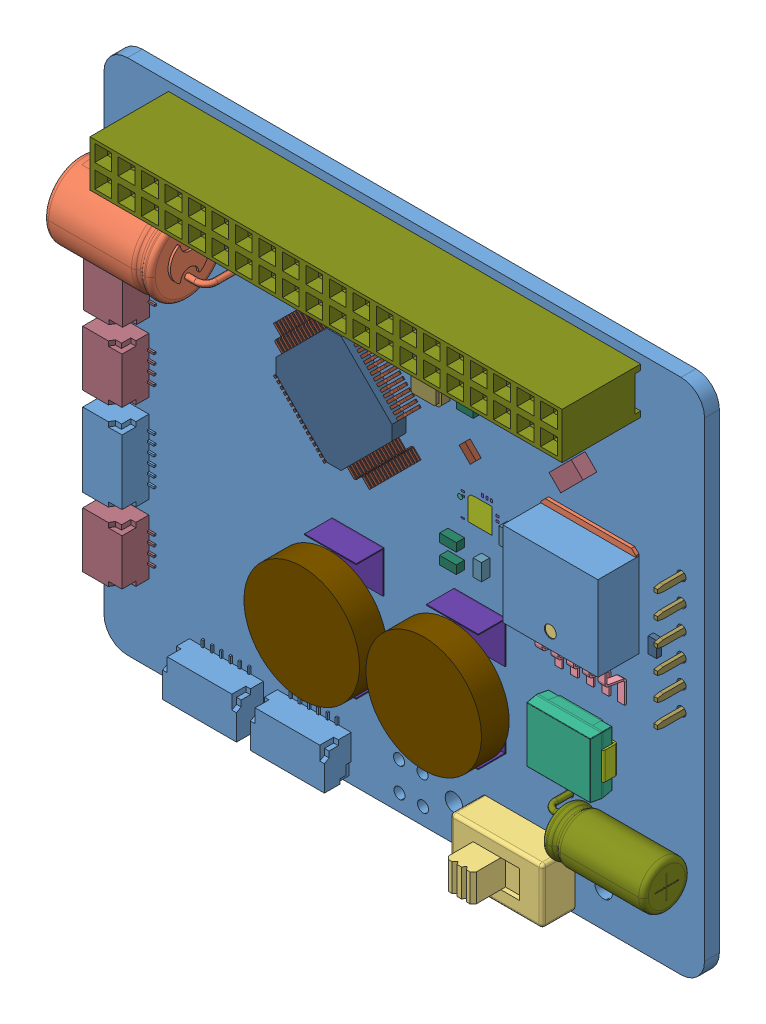
SolidWorks assembly FC_PiHat_REV1, configuration Default. Lengths in mm.
Overall size (65 56 12.01).
297 component instances, 38 part files, 0 mates.
Components (placement in the parent):
- FC_PiHat_REV1.step-1: FC_PiHat_REV1.step [Default] at origin size (65 56 12.01)
  - J7FC_PiHat_REV1.step-1: J7FC_PiHat_REV1.step [Default] at origin size (8 4.95 2.96)
    - SM06B-SRSS-TB.step-1: SM06B-SRSS-TB.step [Default] at (13.3 4.6 -0.3) x (1 0 0) z (0 -1 0) size (8 2.96 4.95)
  - C10FC_PiHat_REV1.step-1: C10FC_PiHat_REV1.step [Default] at origin size (13.96 8.06 10.04)
    - User_Library-Cap_electro_8x11_5x3_5mm_RA.step-1: User_Library-Cap_electro_8x11_5x3_5mm_RA.step [Default] at (13.5254 44.5 4) x (0 1 0) z (0 0 1) size (8.06 13.96 10.04)
  - J11FC_PiHat_REV1.step-1: J11FC_PiHat_REV1.step [Default] at origin size (10 6 9.8)
    - User_Library-EG1940-ND.step-1: User_Library-EG1940-ND.step [Default] at (40.9499 0.2249 0) x (1 0 0) z (0 0 1) size (10 6 9.8)
  - D4FC_PiHat_REV1.step-1: D4FC_PiHat_REV1.step [Default] at origin size (3.4 2.8 1.85)
    - User_Library-RGB_LED_Zwart_ASMT-YTC2-0AA02.step-1: User_Library-RGB_LED_Zwart_ASMT-YTC2-0AA02.step [Default] at (2.2908 8.9737 -1.6023) x (-1 0 0) z (0 -1 0) size (3.4 1.85 2.8)
      - Pootje_RGB_LED.step-1: Pootje_RGB_LED.step [Default] at (-0.3594 -0.1975 0.3238) size (0.9 1.1 0.5)
      - ASMT-YTC2-0AA02.step-1: ASMT-YTC2-0AA02.step [Default] at (-2.6594 -0.3475 0.5738) size (3 1.8 2.8)
      - Pootje_RGB_LED.step-2: Pootje_RGB_LED.step [Default] at (-0.3594 -0.1975 -0.5762) size (0.9 1.1 0.5)
      - Pootje_RGB_LED.step-3: Pootje_RGB_LED.step [Default] at (-0.3594 -0.1975 -1.4762) size (0.9 1.1 0.5)
      - Pootje_RGB_LED.step-4: Pootje_RGB_LED.step [Default] at (-1.9594 -0.1975 -1.9762) x (-1 0 0) z (0 0 -1) size (0.9 1.1 0.5)
      - Pootje_RGB_LED.step-5: Pootje_RGB_LED.step [Default] at (-1.9594 -0.1975 -1.0762) x (-1 0 0) z (0 0 -1) size (0.9 1.1 0.5)
      - Pootje_RGB_LED.step-6: Pootje_RGB_LED.step [Default] at (-1.9594 -0.1975 -0.1762) x (-1 0 0) z (0 0 -1) size (0.9 1.1 0.5)
  - D3FC_PiHat_REV1.step-1: D3FC_PiHat_REV1.step [Default] at origin size (3.4 2.8 1.85)
    - User_Library-RGB_LED_Zwart_ASMT-YTC2-0AA02.step-1: User_Library-RGB_LED_Zwart_ASMT-YTC2-0AA02.step [Default] at (2.3908 45.4737 -1.6023) x (-1 0 0) z (0 -1 0) size (3.4 1.85 2.8)
      - Pootje_RGB_LED.step-1: Pootje_RGB_LED.step [Default] at (-0.3594 -0.1975 0.3238) size (0.9 1.1 0.5)
      - ASMT-YTC2-0AA02.step-1: ASMT-YTC2-0AA02.step [Default] at (-2.6594 -0.3475 0.5738) size (3 1.8 2.8)
      - Pootje_RGB_LED.step-2: Pootje_RGB_LED.step [Default] at (-0.3594 -0.1975 -0.5762) size (0.9 1.1 0.5)
      - Pootje_RGB_LED.step-3: Pootje_RGB_LED.step [Default] at (-0.3594 -0.1975 -1.4762) size (0.9 1.1 0.5)
      - Pootje_RGB_LED.step-4: Pootje_RGB_LED.step [Default] at (-1.9594 -0.1975 -1.9762) x (-1 0 0) z (0 0 -1) size (0.9 1.1 0.5)
      - Pootje_RGB_LED.step-5: Pootje_RGB_LED.step [Default] at (-1.9594 -0.1975 -1.0762) x (-1 0 0) z (0 0 -1) size (0.9 1.1 0.5)
      - Pootje_RGB_LED.step-6: Pootje_RGB_LED.step [Default] at (-1.9594 -0.1975 -0.1762) x (-1 0 0) z (0 0 -1) size (0.9 1.1 0.5)
  - D2FC_PiHat_REV1.step-1: D2FC_PiHat_REV1.step [Default] at origin size (3.4 2.8 1.85)
    - User_Library-RGB_LED_Zwart_ASMT-YTC2-0AA02.step-1: User_Library-RGB_LED_Zwart_ASMT-YTC2-0AA02.step [Default] at (62.5092 10.7763 -1.6023) x (1 0 0) z (0 1 0) size (3.4 1.85 2.8)
      - Pootje_RGB_LED.step-1: Pootje_RGB_LED.step [Default] at (-0.3594 -0.1975 0.3238) size (0.9 1.1 0.5)
      - ASMT-YTC2-0AA02.step-1: ASMT-YTC2-0AA02.step [Default] at (-2.6594 -0.3475 0.5738) size (3 1.8 2.8)
      - Pootje_RGB_LED.step-2: Pootje_RGB_LED.step [Default] at (-0.3594 -0.1975 -0.5762) size (0.9 1.1 0.5)
      - Pootje_RGB_LED.step-3: Pootje_RGB_LED.step [Default] at (-0.3594 -0.1975 -1.4762) size (0.9 1.1 0.5)
      - Pootje_RGB_LED.step-4: Pootje_RGB_LED.step [Default] at (-1.9594 -0.1975 -1.9762) x (-1 0 0) z (0 0 -1) size (0.9 1.1 0.5)
      - Pootje_RGB_LED.step-5: Pootje_RGB_LED.step [Default] at (-1.9594 -0.1975 -1.0762) x (-1 0 0) z (0 0 -1) size (0.9 1.1 0.5)
      - Pootje_RGB_LED.step-6: Pootje_RGB_LED.step [Default] at (-1.9594 -0.1975 -0.1762) x (-1 0 0) z (0 0 -1) size (0.9 1.1 0.5)
  - D1FC_PiHat_REV1.step-1: D1FC_PiHat_REV1.step [Default] at origin size (3.4 2.8 1.85)
    - User_Library-RGB_LED_Zwart_ASMT-YTC2-0AA02.step-1: User_Library-RGB_LED_Zwart_ASMT-YTC2-0AA02.step [Default] at (62.7592 46.4263 -1.6023) x (1 0 0) z (0 1 0) size (3.4 1.85 2.8)
      - Pootje_RGB_LED.step-1: Pootje_RGB_LED.step [Default] at (-0.3594 -0.1975 0.3238) size (0.9 1.1 0.5)
      - ASMT-YTC2-0AA02.step-1: ASMT-YTC2-0AA02.step [Default] at (-2.6594 -0.3475 0.5738) size (3 1.8 2.8)
      - Pootje_RGB_LED.step-2: Pootje_RGB_LED.step [Default] at (-0.3594 -0.1975 -0.5762) size (0.9 1.1 0.5)
      - Pootje_RGB_LED.step-3: Pootje_RGB_LED.step [Default] at (-0.3594 -0.1975 -1.4762) size (0.9 1.1 0.5)
      - Pootje_RGB_LED.step-4: Pootje_RGB_LED.step [Default] at (-1.9594 -0.1975 -1.9762) x (-1 0 0) z (0 0 -1) size (0.9 1.1 0.5)
      - Pootje_RGB_LED.step-5: Pootje_RGB_LED.step [Default] at (-1.9594 -0.1975 -1.0762) x (-1 0 0) z (0 0 -1) size (0.9 1.1 0.5)
      - Pootje_RGB_LED.step-6: Pootje_RGB_LED.step [Default] at (-1.9594 -0.1975 -0.1762) x (-1 0 0) z (0 0 -1) size (0.9 1.1 0.5)
  - S1FC_PiHat_REV1.step-1: S1FC_PiHat_REV1.step [Default] at origin size (4.1 4.1 0.81)
    - 5843174976.step-1: 5843174976.step [Default] at (40.7 32.3 0) size (4.1 4.1 0.81)
      - Body.step-1: Body.step [Default] at (-2.05 -2.05 0)
        - Open_CASCADE_STEP_translator_6.8_14.2.1.x_t-1: Open_CASCADE_STEP_translator_6.8_14.2.1.x_t [Default] at origin
      - Open_CASCADE_STEP_translator_6.8_14.1.step-1: Open_CASCADE_STEP_translator_6.8_14.1.step [Default] at (-2.05 -2.05 0) size (0.52 0.52 0.01)
      - Thermal_Shape.step-1: Thermal_Shape.step [Default] at (-1.3 -1.35 -0.001) size (2.6 2.7 0)
      - Pin_Shape.step-1: Pin_Shape.step [Default] at (-2.05 -1.37 0) size (0.35 0.24 0)
      - Pin_Shape.step-2: Pin_Shape.step [Default] at (2.05 1.37 0) x (-1 0 0) z (0 0 1) size (0.35 0.24 0)
      - Pin_Shape.step-3: Pin_Shape.step [Default] at (-2.05 -0.87 0) size (0.35 0.24 0)
      - Pin_Shape.step-4: Pin_Shape.step [Default] at (2.05 0.87 0) x (-1 0 0) z (0 0 1) size (0.35 0.24 0)
      - Pin_Shape.step-5: Pin_Shape.step [Default] at (-2.05 -0.37 0) size (0.35 0.24 0)
      - Pin_Shape.step-6: Pin_Shape.step [Default] at (2.05 0.37 0) x (-1 0 0) z (0 0 1) size (0.35 0.24 0)
      - Pin_Shape.step-7: Pin_Shape.step [Default] at (-2.05 0.13 0) size (0.35 0.24 0)
      - Pin_Shape.step-8: Pin_Shape.step [Default] at (2.05 -0.13 0) x (-1 0 0) z (0 0 1) size (0.35 0.24 0)
      - Pin_Shape.step-9: Pin_Shape.step [Default] at (-2.05 0.63 0) size (0.35 0.24 0)
      - Pin_Shape.step-10: Pin_Shape.step [Default] at (2.05 -0.63 0) x (-1 0 0) z (0 0 1) size (0.35 0.24 0)
      - Pin_Shape.step-11: Pin_Shape.step [Default] at (-2.05 1.13 0) size (0.35 0.24 0)
      - Pin_Shape.step-12: Pin_Shape.step [Default] at (2.05 -1.13 0) x (-1 0 0) z (0 0 1) size (0.35 0.24 0)
      - Pin_Shape.step-13: Pin_Shape.step [Default] at (-1.13 -2.05 0) x (0 1 0) z (0 0 1) size (0.35 0.24 0)
      - Pin_Shape.step-14: Pin_Shape.step [Default] at (1.13 2.05 0) x (0 -1 0) z (0 0 1) size (0.35 0.24 0)
      - Pin_Shape.step-15: Pin_Shape.step [Default] at (-0.63 -2.05 0) x (0 1 0) z (0 0 1) size (0.35 0.24 0)
      - Pin_Shape.step-16: Pin_Shape.step [Default] at (0.63 2.05 0) x (0 -1 0) z (0 0 1) size (0.35 0.24 0)
      - Pin_Shape.step-17: Pin_Shape.step [Default] at (-0.13 -2.05 0) x (0 1 0) z (0 0 1) size (0.35 0.24 0)
      - Pin_Shape.step-18: Pin_Shape.step [Default] at (0.13 2.05 0) x (0 -1 0) z (0 0 1) size (0.35 0.24 0)
      - Pin_Shape.step-19: Pin_Shape.step [Default] at (0.37 -2.05 0) x (0 1 0) z (0 0 1) size (0.35 0.24 0)
      - Pin_Shape.step-20: Pin_Shape.step [Default] at (-0.37 2.05 0) x (0 -1 0) z (0 0 1) size (0.35 0.24 0)
      - Pin_Shape.step-21: Pin_Shape.step [Default] at (0.87 -2.05 0) x (0 1 0) z (0 0 1) size (0.35 0.24 0)
      - Pin_Shape.step-22: Pin_Shape.step [Default] at (-0.87 2.05 0) x (0 -1 0) z (0 0 1) size (0.35 0.24 0)
      - Pin_Shape.step-23: Pin_Shape.step [Default] at (1.37 -2.05 0) x (0 1 0) z (0 0 1) size (0.35 0.24 0)
      - Pin_Shape.step-24: Pin_Shape.step [Default] at (-1.37 2.05 0) x (0 -1 0) z (0 0 1) size (0.35 0.24 0)
  - R14FC_PiHat_REV1.step-1: R14FC_PiHat_REV1.step [Default] at origin size (1.7 0.9 0.55)
    - 6063442624.step-1: 6063442624.step [Default] at (8.7742 7.9 -2.1523) size (1.7 0.9 0.55)
      - Extruded.step-1: Extruded.step [Default] at origin size (1.7 0.9 0.55)
  - R13FC_PiHat_REV1.step-1: R13FC_PiHat_REV1.step [Default] at origin size (1.7 0.9 0.55)
    - 6063442624.step-1: 6063442624.step [Default] at (8.7742 9.8048 -2.1523) size (1.7 0.9 0.55)
      - Extruded.step-1: Extruded.step [Default] at origin size (1.7 0.9 0.55)
  - R12FC_PiHat_REV1.step-1: R12FC_PiHat_REV1.step [Default] at origin size (1.7 0.9 0.55)
    - 6063442624.step-1: 6063442624.step [Default] at (8.7742 11.7 -2.1523) size (1.7 0.9 0.55)
      - Extruded.step-1: Extruded.step [Default] at origin size (1.7 0.9 0.55)
  - R11FC_PiHat_REV1.step-1: R11FC_PiHat_REV1.step [Default] at origin size (1.7 0.9 0.55)
    - 6063442624.step-1: 6063442624.step [Default] at (9.05 44.4 -2.1523) size (1.7 0.9 0.55)
      - Extruded.step-1: Extruded.step [Default] at origin size (1.7 0.9 0.55)
  - R10FC_PiHat_REV1.step-1: R10FC_PiHat_REV1.step [Default] at origin size (1.7 0.9 0.55)
    - 6063442624.step-1: 6063442624.step [Default] at (9.05 46.3 -2.1523) size (1.7 0.9 0.55)
      - Extruded.step-1: Extruded.step [Default] at origin size (1.7 0.9 0.55)
  - R9FC_PiHat_REV1.step-1: R9FC_PiHat_REV1.step [Default] at origin size (0.9 1.7 0.55)
    - 6063442432.step-1: 6063442432.step [Default] at (59.9 29.7 0) size (0.9 1.7 0.55)
      - Extruded-0.step-1: Extruded-0.step [Default] at origin size (0.9 1.7 0.55)
  - R8FC_PiHat_REV1.step-1: R8FC_PiHat_REV1.step [Default] at origin size (1.7 0.9 0.55)
    - 6063442624.step-1: 6063442624.step [Default] at (9.05 48.2 -2.1523) size (1.7 0.9 0.55)
      - Extruded.step-1: Extruded.step [Default] at origin size (1.7 0.9 0.55)
  - R7FC_PiHat_REV1.step-1: R7FC_PiHat_REV1.step [Default] at origin size (1.84 1.84 0.55)
    - 6063441088.step-1: 6063441088.step [Default] at (39.9 37.9 0) size (1.84 1.84 0.55)
      - Extruded-1.step-1: Extruded-1.step [Default] at origin size (1.84 1.84 0.55)
  - R6FC_PiHat_REV1.step-1: R6FC_PiHat_REV1.step [Default] at origin size (1.7 0.9 0.55)
    - 6063442624.step-1: 6063442624.step [Default] at (56.2 11.8 -2.1523) size (1.7 0.9 0.55)
      - Extruded.step-1: Extruded.step [Default] at origin size (1.7 0.9 0.55)
  - R5FC_PiHat_REV1.step-1: R5FC_PiHat_REV1.step [Default] at origin size (1.7 0.9 0.55)
    - 6063442624.step-1: 6063442624.step [Default] at (56.2 10 -2.1523) size (1.7 0.9 0.55)
      - Extruded.step-1: Extruded.step [Default] at origin size (1.7 0.9 0.55)
  - R4FC_PiHat_REV1.step-1: R4FC_PiHat_REV1.step [Default] at origin size (1.7 0.9 0.55)
    - 6063442624.step-1: 6063442624.step [Default] at (56.2 8.2 -2.1523) size (1.7 0.9 0.55)
      - Extruded.step-1: Extruded.step [Default] at origin size (1.7 0.9 0.55)
  - R3FC_PiHat_REV1.step-1: R3FC_PiHat_REV1.step [Default] at origin size (1.7 0.9 0.55)
    - 6063442624.step-1: 6063442624.step [Default] at (56.8 47.4 -2.1523) size (1.7 0.9 0.55)
      - Extruded.step-1: Extruded.step [Default] at origin size (1.7 0.9 0.55)
  - R2FC_PiHat_REV1.step-1: R2FC_PiHat_REV1.step [Default] at origin size (1.7 0.9 0.55)
    - 6063442624.step-1: 6063442624.step [Default] at (56.8 45.6 -2.1523) size (1.7 0.9 0.55)
      - Extruded.step-1: Extruded.step [Default] at origin size (1.7 0.9 0.55)
  - R1FC_PiHat_REV1.step-1: R1FC_PiHat_REV1.step [Default] at origin size (1.7 0.9 0.55)
    - 6063442624.step-1: 6063442624.step [Default] at (56.8 43.8 -2.1523) size (1.7 0.9 0.55)
      - Extruded.step-1: Extruded.step [Default] at origin size (1.7 0.9 0.55)
  - J8FC_PiHat_REV1.step-1: J8FC_PiHat_REV1.step [Default] at origin size (4.95 8 2.96)
    - SM06B-SRSS-TB.step-1: SM06B-SRSS-TB.step [Default] at (4.55 19.8 -0.3) x (0 -1 0) z (-1 0 0) size (8 2.96 4.95)
  - J6FC_PiHat_REV1.step-1: J6FC_PiHat_REV1.step [Default] at origin size (10.06 15.53 5.7)
    - female_header_a-bl254-ea-g02d.step-1: female_header_a-bl254-ea-g02d.step [Default] at (61.2001 31.0851 -1.6023) x (0 -1 0) z (0 0 -1) size (5.33 10.06 5.7)
    - female_header_a-bl254-ea-g02d.step-2: female_header_a-bl254-ea-g02d.step [Default] at (61.2001 26.0099 -1.6023) x (0 -1 0) z (0 0 -1) size (5.33 10.06 5.7)
    - female_header_a-bl254-ea-g02d.step-3: female_header_a-bl254-ea-g02d.step [Default] at (61.2001 36.2099 -1.6023) x (0 -1 0) z (0 0 -1) size (5.33 10.06 5.7)
  - J4FC_PiHat_REV1.step-1: J4FC_PiHat_REV1.step [Default] at origin size (4.95 6 2.96)
    - SM04B-SRSS-TB.step-1: SM04B-SRSS-TB.step [Default] at (4.55 28.375 -0.3) x (0 -1 0) z (-1 0 0) size (6 2.96 4.95)
  - J3FC_PiHat_REV1.step-1: J3FC_PiHat_REV1.step [Default] at origin size (4.95 6 2.96)
    - SM04B-SRSS-TB.step-1: SM04B-SRSS-TB.step [Default] at (4.55 11.35 -0.3) x (0 -1 0) z (-1 0 0) size (6 2.96 4.95)
  - J2FC_PiHat_REV1.step-1: J2FC_PiHat_REV1.step [Default] at origin size (8 4.95 2.96)
    - SM06B-SRSS-TB.step-1: SM06B-SRSS-TB.step [Default] at (22.8093 4.575 -0.3) x (1 0 0) z (0 -1 0) size (8 2.96 4.95)
  - J1FC_PiHat_REV1.step-1: J1FC_PiHat_REV1.step [Default] at origin size (4.95 6 2.96)
    - SM04B-SRSS-TB.step-1: SM04B-SRSS-TB.step [Default] at (4.625 35.925 -0.3) x (0 -1 0) z (-1 0 0) size (6 2.96 4.95)
  - C4FC_PiHat_REV1.step-1: C4FC_PiHat_REV1.step [Default] at origin size (0.9 1.8 0.9)
    - 6063440896.step-1: 6063440896.step [Default] at (41.3 27.825 0) size (0.9 1.8 0.9)
      - Extruded-2.step-1: Extruded-2.step [Default] at origin size (0.9 1.8 0.9)
  - C3FC_PiHat_REV1.step-1: C3FC_PiHat_REV1.step [Default] at origin size (0.9 1.8 0.9)
    - 6063440896.step-1: 6063440896.step [Default] at (44.1 32.225 0) size (0.9 1.8 0.9)
      - Extruded-2.step-1: Extruded-2.step [Default] at origin size (0.9 1.8 0.9)
  - C2FC_PiHat_REV1.step-1: C2FC_PiHat_REV1.step [Default] at origin size (1.8 0.9 0.9)
    - 6063441280.step-1: 6063441280.step [Default] at (38.125 28.8 0) size (1.8 0.9 0.9)
      - Extruded-3.step-1: Extruded-3.step [Default] at origin size (1.8 0.9 0.9)
  - C1FC_PiHat_REV1.step-1: C1FC_PiHat_REV1.step [Default] at origin size (1.8 0.9 0.9)
    - 6063441280.step-1: 6063441280.step [Default] at (38.125 26.7 0) size (1.8 0.9 0.9)
      - Extruded-3.step-1: Extruded-3.step [Default] at origin size (1.8 0.9 0.9)
  - J5FC_PiHat_REV1.step-1: J5FC_PiHat_REV1.step [Default] at origin size (51.1 5 11.1)
    - User_Library-Header_2x20_2_54mm.step-1: User_Library-Header_2x20_2_54mm.step [Default] at (56.6601 52.5601 0) x (1 0 0) z (0 -1 0) size (51.1 11.1 5)
  - L2FC_PiHat_REV1.step-1: L2FC_PiHat_REV1.step [Default] at origin size (12.5 12.7 6.1)
    - 5843174592.step-1: 5843174592.step [Default] at (40.7 17.6 0) x (0 1 0) z (0 0 1) size (12.7 12.5 6.1)
      - pin.step-1: pin.step [Default] at (6.35 2.8 0) x (-1 0 0) z (0 0 1) size (4.5 5.6 3)
        - Open_CASCADE_STEP_translator_6.8_3.3.1.step-1: Open_CASCADE_STEP_translator_6.8_3.3.1.step [Default] at origin size (4.5 5.6 3)
      - pin.step-2: pin.step [Default] at (-6.35 -2.8 0) size (4.5 5.6 3)
        - Open_CASCADE_STEP_translator_6.8_3.3.1.step-1: Open_CASCADE_STEP_translator_6.8_3.3.1.step [Default] at origin size (4.5 5.6 3)
      - Body.step-1: Body.step [Default] at (0 0 0.1)
        - Open_CASCADE_STEP_translator_6.8_14.2.1.x_t-1: Open_CASCADE_STEP_translator_6.8_14.2.1.x_t [Default] at origin
      - cylinder.step-1: cylinder.step [Default] at (0 0 0.1) size (12.5 12.5 3)
  - U3FC_PiHat_REV1.step-1: U3FC_PiHat_REV1.step [Default] at origin size (10.3 15.24 4.47)
    - 5843175168.step-1: 5843175168.step [Default] at (52.775 32.425 0) x (0 1 0) z (0 0 1) size (15.24 10.3 4.47)
      - Body-1.step-1: Body-1.step [Default] at (-4.575 -5.15 0) size (9.15 10.3 4.47)
        - Open_CASCADE_STEP_translator_6.8_42.2.1.step-1: Open_CASCADE_STEP_translator_6.8_42.2.1.step [Default] at origin size (9.15 10.3 4.47)
      - tab.step-1: tab.step [Default] at (-4.575 -5.15 0) size (9 10.25 0.35)
        - Open_CASCADE_STEP_translator_6.8_42.8.1.step-1: Open_CASCADE_STEP_translator_6.8_42.8.1.step [Default] at origin size (9 10.25 0.35)
      - Open_CASCADE_STEP_translator_6.8_42.1.step-1: Open_CASCADE_STEP_translator_6.8_42.1.step [Default] at (-4.575 -5.15 0) size (1.3 1.3 0.01)
      - Lead.step-1: Lead.step [Default] at (-4.575 -3.4 0) x (-1 0 0) z (0 0 1) size (5.46 0.75 2.33)
      - Lead.step-2: Lead.step [Default] at (-4.575 -1.7 0) x (-1 0 0) z (0 0 1) size (5.46 0.75 2.33)
      - Lead.step-3: Lead.step [Default] at (-4.575 0 0) x (-1 0 0) z (0 0 1) size (5.46 0.75 2.33)
      - Lead.step-4: Lead.step [Default] at (-4.575 1.7 0) x (-1 0 0) z (0 0 1) size (5.46 0.75 2.33)
      - Lead.step-5: Lead.step [Default] at (-4.575 3.4 0) x (-1 0 0) z (0 0 1) size (5.46 0.75 2.33)
    - 5843175168-4.step-1: 5843175168-4.step [Default] at (52.775 32.425 0) x (0 1 0) z (0 0 1) size (2.73 0.75 0.2)
  - D6FC_PiHat_REV1.step-1: D6FC_PiHat_REV1.step [Default] at origin size (7.55 6.23 2.62)
    - 5843175552.step-1: 5843175552.step [Default] at (51.8001 16.8001 0) x (1 0 0) z (0 0 1) size (7.55 6.22 2.62)
      - Body-2.step-1: Body-2.step [Default] at (-3.555 -3.11 0.25) size (7.12 6.22 2.47)
        - Open_CASCADE_STEP_translator_6.8_45.1.1.step-1: Open_CASCADE_STEP_translator_6.8_45.1.1.step [Default] at origin size (7.12 6.22 2.47)
      - Lead-5.step-1: Lead-5.step [Default] at (2.635 0 0) size (1.14 3 1.53)
      - Lead-5.step-2: Lead-5.step [Default] at (-2.635 0 0) x (-1 0 0) z (0 0 1) size (1.14 3 1.53)
  - U2FC_PiHat_REV1.step-1: U2FC_PiHat_REV1.step [Default] at origin size (3.98 3.97 1)
    - 5843176128.step-1: 5843176128.step [Default] at (49.3313 45.4354 0) x (0.707107 -0.707107 0) z (0 0 1) size (2.8 2.91 1)
      - Body-3.step-1: Body-3.step [Default] at (-0.8 -1.45 0) size (1.6 2.91 0.95)
        - Open_CASCADE_STEP_translator_6.8_3.1.1.step-1: Open_CASCADE_STEP_translator_6.8_3.1.1.step [Default] at origin size (1.6 2.91 0.95)
      - Leader.step-1: Leader.step [Default] at (-0.8 -0.95 0) x (-1 0 0) z (0 0 1) size (0.6 0.5 0.57)
      - Leader.step-2: Leader.step [Default] at (-0.8 0 0) x (-1 0 0) z (0 0 1) size (0.6 0.5 0.57)
      - Leader.step-3: Leader.step [Default] at (-0.8 0.95 0) x (-1 0 0) z (0 0 1) size (0.6 0.5 0.57)
      - Leader.step-4: Leader.step [Default] at (0.8 -0.95 0) size (0.6 0.5 0.57)
      - Leader.step-5: Leader.step [Default] at (0.8 0.95 0) size (0.6 0.5 0.57)
  - U1FC_PiHat_REV1.step-1: U1FC_PiHat_REV1.step [Default] at origin size (18.98 19.05 1.5)
    - 5843174208.step-1: 5843174208.step [Default] at (26.375 36.65 0) x (-0.707107 -0.707107 0) z (0 0 1) size (14.7 14.7 1.5)
      - Body-4.step-1: Body-4.step [Default] at (-5 -5 0) size (10 10 1.5)
        - Open_CASCADE_STEP_translator_6.8_6.1.1.step-1: Open_CASCADE_STEP_translator_6.8_6.1.1.step [Default] at origin size (10 10 1.5)
      - Leader-6.step-1: Leader-6.step [Default] at (-5 -3.75 0) x (-1 0 0) z (0 0 1) size (2.35 0.27 0.85)
      - Leader-6.step-2: Leader-6.step [Default] at (-3.75 5 0) x (0 1 0) z (0 0 1) size (2.35 0.27 0.85)
      - Leader-6.step-3: Leader-6.step [Default] at (5 -3.75 0) size (2.35 0.27 0.85)
      - Leader-6.step-4: Leader-6.step [Default] at (-3.75 -5 0) x (0 -1 0) z (0 0 1) size (2.35 0.27 0.85)
      - Leader-6.step-5: Leader-6.step [Default] at (-5 -3.25 0) x (-1 0 0) z (0 0 1) size (2.35 0.27 0.85)
      - Leader-6.step-6: Leader-6.step [Default] at (-3.25 5 0) x (0 1 0) z (0 0 1) size (2.35 0.27 0.85)
      - Leader-6.step-7: Leader-6.step [Default] at (5 -3.25 0) size (2.35 0.27 0.85)
      - Leader-6.step-8: Leader-6.step [Default] at (-3.25 -5 0) x (0 -1 0) z (0 0 1) size (2.35 0.27 0.85)
      - Leader-6.step-9: Leader-6.step [Default] at (-5 -2.75 0) x (-1 0 0) z (0 0 1) size (2.35 0.27 0.85)
      - Leader-6.step-10: Leader-6.step [Default] at (-2.75 5 0) x (0 1 0) z (0 0 1) size (2.35 0.27 0.85)
      - Leader-6.step-11: Leader-6.step [Default] at (5 -2.75 0) size (2.35 0.27 0.85)
      - Leader-6.step-12: Leader-6.step [Default] at (-2.75 -5 0) x (0 -1 0) z (0 0 1) size (2.35 0.27 0.85)
      - Leader-6.step-13: Leader-6.step [Default] at (-5 -2.25 0) x (-1 0 0) z (0 0 1) size (2.35 0.27 0.85)
      - Leader-6.step-14: Leader-6.step [Default] at (-2.25 5 0) x (0 1 0) z (0 0 1) size (2.35 0.27 0.85)
      - Leader-6.step-15: Leader-6.step [Default] at (5 -2.25 0) size (2.35 0.27 0.85)
      - Leader-6.step-16: Leader-6.step [Default] at (-2.25 -5 0) x (0 -1 0) z (0 0 1) size (2.35 0.27 0.85)
      - Leader-6.step-17: Leader-6.step [Default] at (-5 -1.75 0) x (-1 0 0) z (0 0 1) size (2.35 0.27 0.85)
      - Leader-6.step-18: Leader-6.step [Default] at (-1.75 5 0) x (0 1 0) z (0 0 1) size (2.35 0.27 0.85)
      - Leader-6.step-19: Leader-6.step [Default] at (5 -1.75 0) size (2.35 0.27 0.85)
      - Leader-6.step-20: Leader-6.step [Default] at (-1.75 -5 0) x (0 -1 0) z (0 0 1) size (2.35 0.27 0.85)
      - Leader-6.step-21: Leader-6.step [Default] at (-5 -1.25 0) x (-1 0 0) z (0 0 1) size (2.35 0.27 0.85)
      - Leader-6.step-22: Leader-6.step [Default] at (-1.25 5 0) x (0 1 0) z (0 0 1) size (2.35 0.27 0.85)
      - Leader-6.step-23: Leader-6.step [Default] at (5 -1.25 0) size (2.35 0.27 0.85)
      - Leader-6.step-24: Leader-6.step [Default] at (-1.25 -5 0) x (0 -1 0) z (0 0 1) size (2.35 0.27 0.85)
      - Leader-6.step-25: Leader-6.step [Default] at (-5 -0.75 0) x (-1 0 0) z (0 0 1) size (2.35 0.27 0.85)
      - Leader-6.step-26: Leader-6.step [Default] at (-0.75 5 0) x (0 1 0) z (0 0 1) size (2.35 0.27 0.85)
      - Leader-6.step-27: Leader-6.step [Default] at (5 -0.75 0) size (2.35 0.27 0.85)
      - Leader-6.step-28: Leader-6.step [Default] at (-0.75 -5 0) x (0 -1 0) z (0 0 1) size (2.35 0.27 0.85)
      - Leader-6.step-29: Leader-6.step [Default] at (-5 -0.25 0) x (-1 0 0) z (0 0 1) size (2.35 0.27 0.85)
      - Leader-6.step-30: Leader-6.step [Default] at (-0.25 5 0) x (0 1 0) z (0 0 1) size (2.35 0.27 0.85)
      - Leader-6.step-31: Leader-6.step [Default] at (5 -0.25 0) size (2.35 0.27 0.85)
      - Leader-6.step-32: Leader-6.step [Default] at (-0.25 -5 0) x (0 -1 0) z (0 0 1) size (2.35 0.27 0.85)
      - Leader-6.step-33: Leader-6.step [Default] at (-5 0.25 0) x (-1 0 0) z (0 0 1) size (2.35 0.27 0.85)
      - Leader-6.step-34: Leader-6.step [Default] at (0.25 5 0) x (0 1 0) z (0 0 1) size (2.35 0.27 0.85)
      - Leader-6.step-35: Leader-6.step [Default] at (5 0.25 0) size (2.35 0.27 0.85)
      - Leader-6.step-36: Leader-6.step [Default] at (0.25 -5 0) x (0 -1 0) z (0 0 1) size (2.35 0.27 0.85)
      - Leader-6.step-37: Leader-6.step [Default] at (-5 0.75 0) x (-1 0 0) z (0 0 1) size (2.35 0.27 0.85)
      - Leader-6.step-38: Leader-6.step [Default] at (0.75 5 0) x (0 1 0) z (0 0 1) size (2.35 0.27 0.85)
      - Leader-6.step-39: Leader-6.step [Default] at (5 0.75 0) size (2.35 0.27 0.85)
      - Leader-6.step-40: Leader-6.step [Default] at (0.75 -5 0) x (0 -1 0) z (0 0 1) size (2.35 0.27 0.85)
      - Leader-6.step-41: Leader-6.step [Default] at (-5 1.25 0) x (-1 0 0) z (0 0 1) size (2.35 0.27 0.85)
      - Leader-6.step-42: Leader-6.step [Default] at (1.25 5 0) x (0 1 0) z (0 0 1) size (2.35 0.27 0.85)
      - Leader-6.step-43: Leader-6.step [Default] at (5 1.25 0) size (2.35 0.27 0.85)
      - Leader-6.step-44: Leader-6.step [Default] at (1.25 -5 0) x (0 -1 0) z (0 0 1) size (2.35 0.27 0.85)
      - Leader-6.step-45: Leader-6.step [Default] at (-5 1.75 0) x (-1 0 0) z (0 0 1) size (2.35 0.27 0.85)
      - Leader-6.step-46: Leader-6.step [Default] at (1.75 5 0) x (0 1 0) z (0 0 1) size (2.35 0.27 0.85)
      - Leader-6.step-47: Leader-6.step [Default] at (5 1.75 0) size (2.35 0.27 0.85)
      - Leader-6.step-48: Leader-6.step [Default] at (1.75 -5 0) x (0 -1 0) z (0 0 1) size (2.35 0.27 0.85)
      - Leader-6.step-49: Leader-6.step [Default] at (-5 2.25 0) x (-1 0 0) z (0 0 1) size (2.35 0.27 0.85)
      - Leader-6.step-50: Leader-6.step [Default] at (2.25 5 0) x (0 1 0) z (0 0 1) size (2.35 0.27 0.85)
      - Leader-6.step-51: Leader-6.step [Default] at (5 2.25 0) size (2.35 0.27 0.85)
      - Leader-6.step-52: Leader-6.step [Default] at (2.25 -5 0) x (0 -1 0) z (0 0 1) size (2.35 0.27 0.85)
      - Leader-6.step-53: Leader-6.step [Default] at (-5 2.75 0) x (-1 0 0) z (0 0 1) size (2.35 0.27 0.85)
      - Leader-6.step-54: Leader-6.step [Default] at (2.75 5 0) x (0 1 0) z (0 0 1) size (2.35 0.27 0.85)
      - Leader-6.step-55: Leader-6.step [Default] at (5 2.75 0) size (2.35 0.27 0.85)
      - Leader-6.step-56: Leader-6.step [Default] at (2.75 -5 0) x (0 -1 0) z (0 0 1) size (2.35 0.27 0.85)
      - Leader-6.step-57: Leader-6.step [Default] at (-5 3.25 0) x (-1 0 0) z (0 0 1) size (2.35 0.27 0.85)
      - Leader-6.step-58: Leader-6.step [Default] at (3.25 5 0) x (0 1 0) z (0 0 1) size (2.35 0.27 0.85)
      - Leader-6.step-59: Leader-6.step [Default] at (5 3.25 0) size (2.35 0.27 0.85)
      - Leader-6.step-60: Leader-6.step [Default] at (3.25 -5 0) x (0 -1 0) z (0 0 1) size (2.35 0.27 0.85)
      - Leader-6.step-61: Leader-6.step [Default] at (-5 3.75 0) x (-1 0 0) z (0 0 1) size (2.35 0.27 0.85)
      - Leader-6.step-62: Leader-6.step [Default] at (3.75 5 0) x (0 1 0) z (0 0 1) size (2.35 0.27 0.85)
      - Leader-6.step-63: Leader-6.step [Default] at (5 3.75 0) size (2.35 0.27 0.85)
      - Leader-6.step-64: Leader-6.step [Default] at (3.75 -5 0) x (0 -1 0) z (0 0 1) size (2.35 0.27 0.85)
  - R17FC_PiHat_REV1.step-1: R17FC_PiHat_REV1.step [Default] at origin size (0.9 1.7 0.55)
    - 6063442432.step-1: 6063442432.step [Default] at (29.2 5.9 -2.1523) size (0.9 1.7 0.55)
      - Extruded-0.step-1: Extruded-0.step [Default] at origin size (0.9 1.7 0.55)
  - R15FC_PiHat_REV1.step-1: R15FC_PiHat_REV1.step [Default] at origin size (0.9 1.7 0.55)
    - 6063442432.step-1: 6063442432.step [Default] at (26.8 5.9 -2.1523) size (0.9 1.7 0.55)
      - Extruded-0.step-1: Extruded-0.step [Default] at origin size (0.9 1.7 0.55)
  - Q1FC_PiHat_REV1.step-1: Q1FC_PiHat_REV1.step [Default] at origin size (3.2 5 1.35)
    - User_Library-445-CRYTAL-SMD.step-1: User_Library-445-CRYTAL-SMD.step [Default] at (37.4671 49.9363 0.0126) x (0 1 0) z (1 0 0) size (5 1.35 3.2)
  - L3FC_PiHat_REV1.step-1: L3FC_PiHat_REV1.step [Default] at origin size (12.5 12.7 6.1)
    - 5843174592.step-1: 5843174592.step [Default] at (27.5 17.6 0) x (0 1 0) z (0 0 1) size (12.7 12.5 6.1)
      - pin.step-1: pin.step [Default] at (6.35 2.8 0) x (-1 0 0) z (0 0 1) size (4.5 5.6 3)
        - Open_CASCADE_STEP_translator_6.8_3.3.1.step-1: Open_CASCADE_STEP_translator_6.8_3.3.1.step [Default] at origin size (4.5 5.6 3)
      - pin.step-2: pin.step [Default] at (-6.35 -2.8 0) size (4.5 5.6 3)
        - Open_CASCADE_STEP_translator_6.8_3.3.1.step-1: Open_CASCADE_STEP_translator_6.8_3.3.1.step [Default] at origin size (4.5 5.6 3)
      - Body.step-1: Body.step [Default] at (0 0 0.1)
        - Open_CASCADE_STEP_translator_6.8_14.2.1.x_t-1: Open_CASCADE_STEP_translator_6.8_14.2.1.x_t [Default] at origin
      - cylinder.step-1: cylinder.step [Default] at (0 0 0.1) size (12.5 12.5 3)
  - L1FC_PiHat_REV1.step-1: L1FC_PiHat_REV1.step [Default] at origin size (3.68 3.68 1.5)
    - 6063441856.step-1: 6063441856.step [Default] at (51.5 42 0) size (3.68 3.68 1.5)
      - Extruded-7.step-1: Extruded-7.step [Default] at origin size (3.68 3.68 1.5)
  - D7FC_PiHat_REV1.step-1: D7FC_PiHat_REV1.step [Default] at origin size (0.8 1.6 0.75)
    - 6063441664.step-1: 6063441664.step [Default] at (29.2 2.1 -2.3523) size (0.8 1.2 0.75)
      - Extruded-8.step-1: Extruded-8.step [Default] at origin size (0.8 1.2 0.75)
    - 6063441472.step-1: 6063441472.step [Default] at (29.2 2.8 -2.3523) size (0.8 0.2 0.75)
      - Extruded-9.step-1: Extruded-9.step [Default] at origin size (0.8 0.2 0.75)
    - 6063441472.step-2: 6063441472.step [Default] at (29.2 1.4 -2.3523) size (0.8 0.2 0.75)
      - Extruded-9.step-1: Extruded-9.step [Default] at origin size (0.8 0.2 0.75)
  - D5FC_PiHat_REV1.step-1: D5FC_PiHat_REV1.step [Default] at origin size (0.8 1.6 0.75)
    - 6063441664.step-1: 6063441664.step [Default] at (26.8 2.075 -2.3523) size (0.8 1.2 0.75)
      - Extruded-8.step-1: Extruded-8.step [Default] at origin size (0.8 1.2 0.75)
    - 6063441472.step-1: 6063441472.step [Default] at (26.8 2.775 -2.3523) size (0.8 0.2 0.75)
      - Extruded-9.step-1: Extruded-9.step [Default] at origin size (0.8 0.2 0.75)
    - 6063441472.step-2: 6063441472.step [Default] at (26.8 1.375 -2.3523) size (0.8 0.2 0.75)
      - Extruded-9.step-1: Extruded-9.step [Default] at origin size (0.8 0.2 0.75)
  - C9FC_PiHat_REV1.step-1: C9FC_PiHat_REV1.step [Default] at origin size (13.46 5.06 8.54)
    - User_Library-Cap_electro_5x11x2mm_RA.step-1: User_Library-Cap_electro_5x11x2mm_RA.step [Default] at (51.885 9.9755 2.5) x (0 -1 0) z (0 0 1) size (5.06 13.46 8.54)
  - C8FC_PiHat_REV1.step-1: C8FC_PiHat_REV1.step [Default] at origin size (1.91 1.91 0.9)
    - 6063442048.step-1: 6063442048.step [Default] at (47.1 43.3857 0) size (1.91 1.91 0.9)
      - Extruded-10.step-1: Extruded-10.step [Default] at origin size (1.91 1.91 0.9)
  - C7FC_PiHat_REV1.step-1: C7FC_PiHat_REV1.step [Default] at origin size (1.91 1.91 0.9)
    - 6063442240.step-1: 6063442240.step [Default] at (45.7 46.4 0) size (1.91 1.91 0.9)
      - Extruded-11.step-1: Extruded-11.step [Default] at origin size (1.91 1.91 0.9)
  - C6FC_PiHat_REV1.step-1: C6FC_PiHat_REV1.step [Default] at origin size (1.8 0.9 0.9)
    - 6063441280.step-1: 6063441280.step [Default] at (39.9535 42.2416 0) size (1.8 0.9 0.9)
      - Extruded-3.step-1: Extruded-3.step [Default] at origin size (1.8 0.9 0.9)
  - C5FC_PiHat_REV1.step-1: C5FC_PiHat_REV1.step [Default] at origin size (1.8 0.9 0.9)
    - 6063441280.step-1: 6063441280.step [Default] at (39.9535 44.9915 0) size (1.8 0.9 0.9)
      - Extruded-3.step-1: Extruded-3.step [Default] at origin size (1.8 0.9 0.9)
  - BoardFC_PiHat_REV1.step-1: BoardFC_PiHat_REV1.step [Default] at origin size (65 56 1.6)
